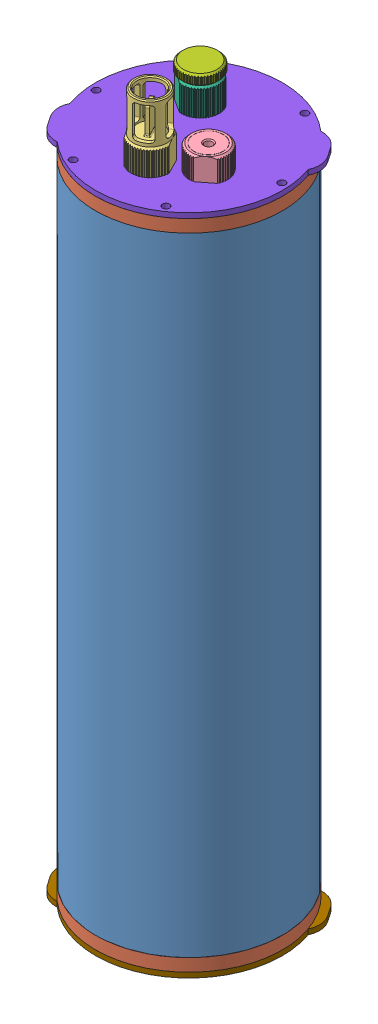
SolidWorks assembly BRPT_v1, configuration Default. Lengths in mm.
Overall size (209.76 357.59 319.54).
47 component instances, 19 part files, 28 mates.
Components (placement in the parent):
- 3in series housing-1: 3in series housing [Default] at (162.5946 57.9765 268.4972) size (88.9 298.45 88.9)
- 3in series Oring flange-1: 3in series Oring flange [Default] at (162.5946 335.4265 268.4972) x (-0.99734 0 0.072895) z (0 -1 0) size (88.9 88.9 27.11)
- 3in series Oring flange-2: 3in series Oring flange [Default] at (162.5946 78.9765 268.4972) x (0.99734 0 -0.072895) z (0 1 0) size (88.9 88.9 27.11)
- CELSIUS-TEMPERATURE-SENSOR-ASSEMBLY-X1-1: CELSIUS-TEMPERATURE-SENSOR-ASSEMBLY-X1 [Default] at (122.5922 326.5947 279.9307) x (0.457003 0 0.889465) z (0 1 0) size (18 16 56.58)
- BAR30-SENSOR-ASSEMBLY-R1-1: BAR30-SENSOR-ASSEMBLY-R1 [Default] at (177.0309 360.3608 268.6158) x (-0.789833 0 0.613322) z (0 1 0) size (18 16 37.53)
- PENETRATOR-M-NUT-10-8-R2-1: PENETRATOR-M-NUT-10-8-R2 [Default] at (151.3587 362.4265 251.9517) x (0.587103 0 -0.809513) z (0 -1 0) size (18 16 9.22)
- VENT-M-BOLT-10-25-A-R4-1: VENT-M-BOLT-10-25-A-R4 [94036A625] at (151.3587 363.5765 251.9517) x (0.845284 0 0.534318) z (0 1 0) size (18 16 39.53)
- VENT-M-PLUG-10-A-R3-1: VENT-M-PLUG-10-A-R3 [Default] at (151.3587 367.5765 251.9517) x (-0.985482 0 -0.169779) z (0 -1 0) size (18 17.99 20.15)
- PENETRATOR-M-NUT-10-8-R2-2: PENETRATOR-M-NUT-10-8-R2 [Default] at (180.598 354.4265 277.208) x (-0.220712 0 -0.975339) z (0 1 0) size (18 16 9.22)
- PENETRATOR-M-NUT-10-8-R2-3: PENETRATOR-M-NUT-10-8-R2 [Default] at (164.0525 362.4265 288.444) x (-0.986467 0 -0.16396) z (0 -1 0) size (18 16 9.22)
- 3in series end cap 3 holes-1: 3in series end cap 3 holes [Default] at (162.5946 362.4265 268.4972) x (-0.827274 0 0.561799) z (-0.561799 0 -0.827274) size (96 2.4 88.9)
- 3in series end cap-2: 3in series end cap [Default] at (162.5946 49.5765 268.4972) x (-0.827274 0 0.561799) z (-0.561799 0 -0.827274) size (96 2.4 88.9)
- Battery holder-1: Battery holder [Default] at (88.5633 90.8064 358.6088) x (-0.32029 0 -0.94732) z (0.94732 0 -0.32029) size (98.62 218.61 98.22)
  - battery holder v2-1: battery holder v2 [Default] at (61.653 68.5201 98.9932) size (71.12 137.5 69.24)
  - 2600mAh Battery-1: 2600mAh Battery [Default] at (86.0749 4.0582 84.8932) x (-0.71885 0 -0.695165) z (0.695165 0 -0.71885) size (18 65 18) (hidden)
  - 2600mAh Battery-2: 2600mAh Battery [Default] at (86.0749 134.0582 84.8932) x (0.792584 0 -0.609763) z (-0.609763 0 -0.792584) size (18 65 18) (hidden)
  - 2600mAh Battery-3: 2600mAh Battery [Default] at (37.231 4.0582 113.0932) size (18 65 18) (hidden)
  - 2600mAh Battery-4: 2600mAh Battery [Default] at (37.231 134.0582 113.0932) x (0.840955 0 0.541105) z (0.541105 0 -0.840955) size (18 65 18) (hidden)
  - 2600mAh Battery-5: 2600mAh Battery [Default] at (61.653 4.0582 127.1932) x (-0.28708 0 -0.957907) z (0.957907 0 -0.28708) size (18 65 18) (hidden)
  - 2600mAh Battery-6: 2600mAh Battery [Default] at (61.653 69.0582 127.1932) x (-0.79051 0 -0.612449) z (0.612449 0 -0.79051) size (18 65 18) (hidden)
  - 2600mAh Battery-7: 2600mAh Battery [Default] at (37.231 4.0582 84.8932) size (18 65 18) (hidden)
  - 2600mAh Battery-8: 2600mAh Battery [Default] at (37.231 69.0582 84.8932) x (-0.486699 0 -0.87357) z (0.87357 0 -0.486699) size (18 65 18) (hidden)
  - Battery holder endcap-1: Battery holder endcap [Default] at (99.0192 180.1854 40.1409) x (-1 0 0) z (0 0 1) size (75.69 15.3 75.69)
    - Battery holder endcap-1: Battery holder endcap [Default] at (37.3662 31.3154 58.8523) size (75.69 14.1 75.69)
    - battery contact 209-2: battery contact 209 [Default] at (9.8065 42.9154 70.2374) x (0 1 0) z (0.5 0 0.866025) size (6.42 12.29 7.92)
    - battery contact 209-3: battery contact 209 [Default] at (33.4462 42.9154 88.4123) x (0 1 0) z (1 0 0) size (6.42 12.29 7.92)
    - battery contact 209-4: battery contact 209 [Default] at (61.0059 42.9154 77.0271) x (0 1 0) z (0.5 0 -0.866025) size (6.42 12.29 7.92)
    - battery contact 209-5: battery contact 209 [Default] at (64.9259 42.9154 47.4671) x (0 1 0) z (-0.5 0 -0.866025) size (6.42 12.29 7.92)
    - battery contact 209-6: battery contact 209 [Default] at (41.2862 42.9154 29.2923) x (0 1 0) z (-1 0 0) size (6.42 12.29 7.92)
    - battery contact 209-7: battery contact 209 [Default] at (13.7265 42.9154 40.6774) x (0 1 0) z (-0.5 0 0.866025) size (6.42 12.29 7.92)
  - Battery holder endcap-2: Battery holder endcap [Default] at (24.2867 -43.1453 40.1409) size (75.69 15.3 75.69)
    - Battery holder endcap-1: Battery holder endcap [Default] at (37.3662 31.3154 58.8523) size (75.69 14.1 75.69)
    - battery contact 209-2: battery contact 209 [Default] at (9.8065 42.9154 70.2374) x (0 1 0) z (0.5 0 0.866025) size (6.42 12.29 7.92)
    - battery contact 209-3: battery contact 209 [Default] at (33.4462 42.9154 88.4123) x (0 1 0) z (1 0 0) size (6.42 12.29 7.92)
    - battery contact 209-4: battery contact 209 [Default] at (61.0059 42.9154 77.0271) x (0 1 0) z (0.5 0 -0.866025) size (6.42 12.29 7.92)
    - battery contact 209-5: battery contact 209 [Default] at (64.9259 42.9154 47.4671) x (0 1 0) z (-0.5 0 -0.866025) size (6.42 12.29 7.92)
    - battery contact 209-6: battery contact 209 [Default] at (41.2862 42.9154 29.2923) x (0 1 0) z (-1 0 0) size (6.42 12.29 7.92)
    - battery contact 209-7: battery contact 209 [Default] at (13.7265 42.9154 40.6774) x (0 1 0) z (-0.5 0 0.866025) size (6.42 12.29 7.92)
  - 92239A100_FLANGED WING NUT-1: 92239A100_FLANGED WING NUT [92239A100] at (61.653 -11.8299 98.9932) x (1 0 0) z (0 1 0) size (22.23 15.88 11.75)
  - 92239A100_FLANGED WING NUT-2: 92239A100_FLANGED WING NUT [92239A100] at (61.653 148.8701 98.9932) x (1 0 0) z (0 -1 0) size (22.23 15.88 11.75)
  - 91565A345_LOW-STRENGTH STEEL THREADED ROD-1: 91565A345_LOW-STRENGTH STEEL THREADED ROD [91565A345] at (61.653 69.9701 98.9932) x (0 1 0) z (-0.704559 0 -0.709645) size (179.29 4.22 4.81)
  - Battery holder spacer-1: Battery holder spacer [Default] at (61.653 -7.5935 98.9932) x (0.5 0 -0.866025) z (-0.866025 0 -0.5) size (71.12 9 73.26)
- Electronics Shelf-2: Electronics Shelf [Default] at (184.5849 247.1362 219.3245) x (0.32029 0 0.94732) z (-0.94732 0 0.32029) size (74.93 81.28 51.4)
  - Electronics Shelf-1: Electronics Shelf [Default] at (39.539 0.3112 46.7413) size (74.93 81.28 33.74)
  - 93505A103_MALE-FEMALE THREADED HEX STANDOFF-2: 93505A103_MALE-FEMALE THREADED HEX STANDOFF [93505A103] at (64.5455 76.1098 32.9301) x (0 0 -1) z (1 0 0) size (17.78 5.5 4.76)
  - 93505A103_MALE-FEMALE THREADED HEX STANDOFF-3: 93505A103_MALE-FEMALE THREADED HEX STANDOFF [93505A103] at (14.5455 76.1098 32.9301) x (0 0 -1) z (1 0 0) size (17.78 5.5 4.76)
  - PCB-1: PCB [Default] at (39.5455 41.1098 28.9613) x (1 0 0) z (0 1 0) size (60 2.54 80)
Mates (geometry in assembly coordinates):
- Coincident1: coincident anti-aligned: circle of 3in series housing-1; circle of 3in series Oring flange-1
- Coincident2: coincident aligned: circle of 3in series housing-1; circle of 3in series Oring flange-2
- Concentric1: concentric anti-aligned: circle of 3in series Oring flange-1; circle of 3in series end cap-1
- Coincident3: coincident anti-aligned: plane of 3in series Oring flange-1 through (118.2629 362.4265 271.7374) normal (0 1 0); plane of 3in series end cap 3 holes-1 through (162.5946 362.4265 268.4972) normal (0 -1 0)
- Concentric2: concentric aligned: circle of 3in series Oring flange-1; circle of 3in series end cap-1
- Concentric3: concentric aligned: circle of 3in series Oring flange-2; circle of 3in series end cap-2
- Coincident6: coincident anti-aligned: plane of 3in series Oring flange-2 through (206.9264 51.9765 265.257) normal (0 -1 0); plane of 3in series end cap-2 through (162.5946 51.9765 268.4972) normal (0 1 0)
- Concentric4: concentric anti-aligned: circle of 3in series Oring flange-2; circle of 3in series end cap-2
- Parallel1: parallel anti-aligned: line of 3in series Oring flange-1 through (118.2629 362.4265 271.7374) axis (0.99734 0 -0.072895); line of 3in series Oring flange-2 through (206.9264 51.9765 265.257) axis (-0.99734 0 0.072895)
- Coincident14: coincident anti-aligned: plane of CELSIUS-TEMPERATURE-SENSOR-ASSEMBLY-X1-1 through (164.0525 364.8265 288.444) normal (0 -1 0); plane of 3in series end cap 3 holes-1 through (162.5946 364.8265 268.4972) normal (0 1 0)
- Coincident15: coincident anti-aligned: plane of VENT-M-BOLT-10-25-A-R4-1 through (151.3587 377.5765 251.9517) normal (0 1 0); plane of VENT-M-PLUG-10-A-R3-1 through (152.1906 377.5765 247.1228) normal (0 -1 0)
- Concentric6: concentric anti-aligned: circle of VENT-M-BOLT-10-25-A-R4-1; circle of VENT-M-PLUG-10-A-R3-1
- Coincident16: coincident anti-aligned: plane of VENT-M-BOLT-10-25-A-R4-1 through (154.2494 364.8265 247.3786) normal (0 -1 0); plane of 3in series end cap 3 holes-1 through (162.5946 364.8265 268.4972) normal (0 1 0)
- Concentric8: concentric anti-aligned: circle of BAR30-SENSOR-ASSEMBLY-R1-1; circle of 3in series end cap 3 holes-1
- Coincident17: coincident anti-aligned: plane of BAR30-SENSOR-ASSEMBLY-R1-1 through (185.2349 364.8265 283.1793) normal (0 -1 0); plane of 3in series end cap 3 holes-1 through (162.5946 364.8265 268.4972) normal (0 1 0)
- Concentric9: concentric anti-aligned: cylinder of PENETRATOR-M-NUT-10-8-R2-1; cylinder of VENT-M-BOLT-10-25-A-R4-1 through (151.3587 338.5765 251.9517) axis (0 1 0) radius 5
- Coincident18: coincident anti-aligned: plane of PENETRATOR-M-NUT-10-8-R2-1 through (151.3587 362.4265 251.9517) normal (0 1 0); plane of 3in series end cap 3 holes-1 through (162.5946 362.4265 268.4972) normal (0 -1 0)
- Concentric10: concentric aligned: circle of BAR30-SENSOR-ASSEMBLY-R1-1; circle of PENETRATOR-M-NUT-10-8-R2-2
- Coincident19: coincident anti-aligned: plane of PENETRATOR-M-NUT-10-8-R2-2 through (180.598 362.4265 277.208) normal (0 1 0); plane of 3in series end cap 3 holes-1 through (162.5946 362.4265 268.4972) normal (0 -1 0)
- Concentric11: concentric anti-aligned: circle of CELSIUS-TEMPERATURE-SENSOR-ASSEMBLY-X1-1; circle of PENETRATOR-M-NUT-10-8-R2-3
- Coincident21: coincident anti-aligned: plane of PENETRATOR-M-NUT-10-8-R2-3 through (164.0525 362.4265 288.444) normal (0 1 0); plane of 3in series end cap 3 holes-1 through (162.5946 362.4265 268.4972) normal (0 -1 0)
- Concentric12: concentric aligned: circle of 3in series housing-1; circle of Battery holder-1/Battery holder endcap-2/Battery holder endcap-1
- Coincident22: coincident anti-aligned: plane of 3in series Oring flange-2 through (162.5946 78.9765 268.4972) normal (0 1 0); plane of Battery holder-1/Battery holder endcap-2/Battery holder endcap-1 through (162.5946 78.9765 268.4972) normal (0 -1 0)
- Concentric13: concentric aligned: circle of CELSIUS-TEMPERATURE-SENSOR-ASSEMBLY-X1-1; circle of 3in series end cap 3 holes-1
- Concentric14: concentric aligned: circle of VENT-M-PLUG-10-A-R3-1; circle of 3in series end cap 3 holes-1
- Parallel7: parallel anti-aligned: plane of Battery holder-1/Battery holder endcap-1/Battery holder endcap-1 through (162.5946 239.6765 268.4972) normal (0 1 0); plane of Electronics Shelf-2/Electronics Shelf-1 through (162.5946 247.4474 268.4972) normal (0 -1 0)
- Concentric16: concentric anti-aligned: circle of Battery holder-1/Battery holder endcap-1/Battery holder endcap-1; circle of Electronics Shelf-2/Electronics Shelf-1
- Parallel8: parallel anti-aligned: plane of Battery holder-1/92239A100_FLANGED WING NUT-2 through (161.4575 240.78 265.7311) normal (-0.94732 0 0.32029); plane of Electronics Shelf-2/Electronics Shelf-1 through (145.7826 328.7274 234.6329) normal (0.94732 0 -0.32029)
